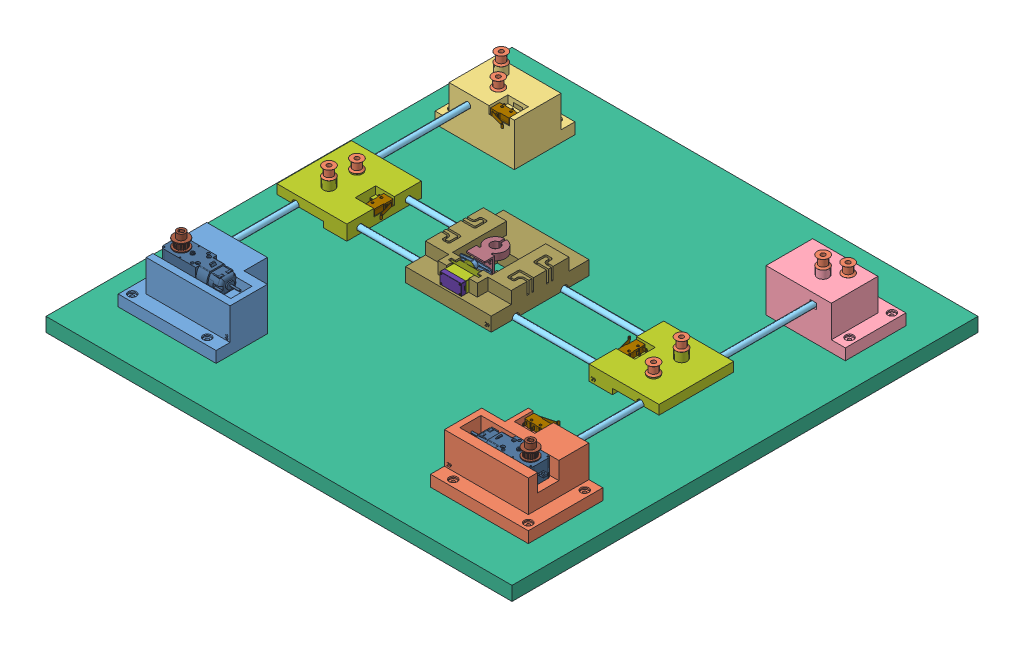
SolidWorks assembly LATEST ASSEMBLY, configuration Default. Lengths in mm.
Overall size (500 85.8 500).
74 component instances, 40 part files, 223 mates.
Components (placement in the parent):
- Stepper LEFT-2: Stepper LEFT [Default] at (56.9106 18.8224 107.4088) x (0 0 1) z (0 1 0) size (80 105 46)
- Stepper Right-1: Stepper Right [Default] at (296.9106 18.8224 42.4088) size (105 46 80)
- EndEffector 2-1: EndEffector 2 [Default] at (-28.0894 18.8224 -267.5912) size (85 56 65)
- EndEffector 1-1: EndEffector 1 [Default] at (384.024 18.8224 -217.5912) x (0 0 1) z (-1 0 0) size (65 54.7 85)
- Shaft-1: Shaft [Default] at (-8.0894 53.8224 -237.5912) x (-0.999824 -0.018749 0) z (-0.018749 0.999824 0) size (6 300 6)
- Shaft-4: Shaft [Default] at (361.9106 53.6724 -237.5912) x (-0.560083 -0.828436 0) z (-0.828436 0.560083 0) size (6 300 6)
- Base-2: Base [Default] at (426.9106 3.8224 -330.0912) size (500 15 500)
- END EFFECTOR 1-1: END EFFECTOR 1 [Default] at (321.9104 53.0886 -32.8378) x (0 0 -1) z (1 -0.000405 0) size (80 26 75)
- LMU-N6-1: LMU-N6 [Default] at (361.9106 53.6724 -72.5878) x (0 1 0) z (-1 0 0) size (12 19 12)
- END EFFECTOR 1-2: END EFFECTOR 1 [Default] at (31.9104 53.2062 -112.8378) x (0 0 1) z (-1 0.000405 0) size (80 26 75)
- LMU-N6-2: LMU-N6 [Default] at (-8.0894 53.8224 -73.0878) x (1 0 0) z (0 -1 0) size (12 19 12)
- Shaft-5: Shaft [Default] at (326.9104 53.0866 -98.8378) x (0.000405 1 0) z (0 0 1) size (6 300 6)
- Shaft-6: Shaft [Default] at (26.9104 53.2082 -46.8378) x (0.000401 0.988771 0.149436) z (0.000061 0.149436 -0.988771) size (6 300 6)
- LMU-N6-3: LMU-N6 [Default] at (167.865 53.151 -98.8378) x (0.000405 1 0) z (0 0 1) size (12 19 12)
- LMU-N6-4: LMU-N6 [Default] at (191.865 53.1413 -46.8378) x (0 0 -1) z (-0.000405 -1 0) size (12 19 12)
- LMU-N6-5: LMU-N6 [Default] at (145.865 53.16 -46.8378) x (0 0 -1) z (-0.000405 -1 0) size (12 19 12)
- A4_paper-1: A4_paper [Default] at (181.5617 18.8224 -76.6394) size (210 0.3 297) (hidden)
- SS_5GL13.step-10: SS_5GL13.step [Default] at (39.2125 58.4032 -68.0878) x (0 0 1) z (0.000405 1 0) size (21.03 22.89 6.4)
- SS_5GL13.step-11: SS_5GL13.step [Default] at (314.6125 58.2916 -77.5878) x (0 0 -1) z (0.000405 1 0) size (21.03 22.89 6.4)
- SS_5GL13.step-12: SS_5GL13.step [Default] at (337.6606 60.0224 50.1088) x (1 0 0) z (0 1 0) size (21.03 22.89 6.4)
- DG01D Motor-10: DG01D Motor [Default] at (-9.0894 55.8224 88.8088) x (-1 0 0) z (0 -1 0) size (79.2 22.5 37.6)
- DG01D Motor-11: DG01D Motor [Default] at (362.9106 46.0224 86.0088) x (1 0 0) z (0 -1 0) size (79.2 22.5 37.6)
- GT2 20T motor-2: GT2 20T motor [Default] at (-9.0894 83.1224 88.8088) x (0.422618 0 0.906308) z (0 1 0) size (16 16 15)
- GT2 20T motor-3: GT2 20T motor [Default] at (362.9106 73.3224 86.0088) x (-0.422618 0 -0.906308) z (0 1 0) size (16 16 15)
- belt Red^LATEST ASSEMBLY-1: belt Red^LATEST ASSEMBLY [Default] at origin (suppressed, hidden, virtual)
- SS_5GL13.step-14: SS_5GL13.step [Default] at (30.6606 60.0224 -225.2912) x (1 0 0) z (0 -1 0) size (21.03 22.89 6.4)
- ENDEFFECTOR-2: ENDEFFECTOR [Default] at (122.3648 52.6695 -125.3378) x (0 0 1) z (-1 0.000405 0) size (105 28 92)
- Pen Holder-2: Pen Holder [Default] at (168.2252 78.3723 -70.9178) x (0 0 1) z (0.000405 1 0) size (32.33 22 45.5)
- servo-3: servo [Default] at (161.2865 54.9158 -21.6708) x (1 -0.000405 0) z (0.000405 1 0) size (38.91 33.08 16.81)
  - servo.STEP-1: servo.STEP [Default] at origin size (38.91 33.08 16.81)
    - gear_sub1.STEP-1: gear_sub1.STEP [Default] at (5.1357 15.652 26.5654) x (-0.68795 0 -0.725758) z (0.725758 0 -0.68795) size (14.38 10.78 14.37)
      - scrow.STEP-1: scrow.STEP [Default] at (3.6352 0.49 7.5429) size (1 10.78 1)
      - spur gear_iso_ISO - Spur gear 0.25M 39T 20PA 1FW ---S39A75H50L1.0N.STEP-1: spur gear_iso_ISO - Spur gear 0.25M 39T 20PA 1FW ---S39A75H50L1.0N.STEP [Default] at (3.6352 0.49 7.5429) x (0 1 0) z (-0.789182 0 0.61416) size (1 10.24 10.25)
      - spur gear_iso_ISO - Spur gear 0.25M 10T 20PA 1.75FW ---S10A75H50L1.0N.STEP-1: spur gear_iso_ISO - Spur gear 0.25M 10T 20PA 1.75FW ---S10A75H50L1.0N.STEP [Default] at (3.6352 1.49 7.5429) x (0 1 0) z (-0.998551 0 0.053813) size (1.75 2.87 3)
    - gear_sub2.STEP-1: gear_sub2.STEP [Default] at (8.1037 16.927 13.0282) x (0.29675 0 0.954955) z (-0.954955 0 0.29675) size (10.78 2.75 10.78)
      - spur gear_iso_ISO - Spur gear 0.25M 39T 20PA 1FW ---S39A75H50L1.0N.STEP-1: spur gear_iso_ISO - Spur gear 0.25M 39T 20PA 1FW ---S39A75H50L1.0N.STEP [Default] at (3.6352 0.59 7.5429) x (0 1 0) z (-0.998551 0 0.053813) size (1 10.24 10.25)
      - spur gear_iso_ISO - Spur gear 0.25M 10T 20PA 1.75FW ---S10A75H50L1.0N.STEP-1: spur gear_iso_ISO - Spur gear 0.25M 10T 20PA 1.75FW ---S10A75H50L1.0N.STEP [Default] at (3.6352 1.59 7.5429) x (0 1 0) z (-0.998551 0 0.053813) size (1.75 2.87 3)
    - gear_sub3.STEP-1: gear_sub3.STEP [Default] at (15.6535 19.4558 12.7337) x (0.175743 0 0.984436) z (-0.984436 0 0.175743) size (10.78 7 10.78)
      - spur gear_iso_ISO - Spur gear 0.25M 39T 20PA 1FW ---S39A75H50L1.0N.STEP-1: spur gear_iso_ISO - Spur gear 0.25M 39T 20PA 1FW ---S39A75H50L1.0N.STEP [Default] at (4.585 -0.5638 8.482) x (0 1 0) z (-0.998551 0 0.053813) size (1 10.24 10.25)
      - spur gear_iso_ISO - Spur gear 0.25M 10T 20PA 6FW ---S10A75H50L1.0N.STEP-1: spur gear_iso_ISO - Spur gear 0.25M 10T 20PA 6FW ---S10A75H50L1.0N.STEP [Default] at (4.585 6.4362 8.482) x (0 -1 0) z (-0.985477 0 0.169808) size (6 2.87 3)
    - DcMotor Emsamblaje Final_Predeterminado.STEP-1: DcMotor Emsamblaje Final_Predeterminado.STEP [Default] at (14.2292 7.0834 18.738) x (0 0 1) z (0 1 0) size (9.11 7.45 12.63)
      - TapaCarcasaDcMotor_Predeterminado.STEP-1: TapaCarcasaDcMotor_Predeterminado.STEP [Default] at origin size (9.07 6.88 5)
      - RondanaDcMotor_Predeterminado.STEP-1: RondanaDcMotor_Predeterminado.STEP [Default] at (0 0 -4.154) x (-0.908878 0.417062 0) z (0 0 1) size (2.73 2.73 1.36)
      - Soportede Cobre_Predeterminado.STEP-1: Soportede Cobre_Predeterminado.STEP [Default] at (-2.4158 -0.0897 0.8236) x (-1 0 0) z (0 0 -1) size (3.11 2.85 3.19)
      - CarcasaDcMotor_Predeterminado.STEP-1: CarcasaDcMotor_Predeterminado.STEP [Default] at (-0.0001 -0.0021 2.4378) size (9.11 7.45 9.44)
      - Arcometalico_Predeterminado.STEP-1: Arcometalico_Predeterminado.STEP [Default] at (0 3.5144 -4.5886) x (1 0 0) z (0 0 -1) size (3.87 0.45 7.17)
      - AislanteDcMotor_Predeterminado.STEP-1: AislanteDcMotor_Predeterminado.STEP [Default] at (-4.0652 -0.1559 -3.4215) x (0.999266 0.038313 0) z (0 0 1) size (2.31 6.27 5.47)
      - AislanteDcMotor_Predeterminado.STEP-2: AislanteDcMotor_Predeterminado.STEP [Default] at (4.0652 -0.1559 8.5785) x (-0.999266 0.038313 0) z (0 0 -1) size (2.31 6.27 5.47)
      - Rondana2DcMotor_Predeterminado.STEP-1: Rondana2DcMotor_Predeterminado.STEP [Default] at (0 0 8.6961) x (-0.478461 0.878109 0) z (0 0 -1) size (2.5 2.5 0.8)
      - Soportede Cobre_Predeterminado.STEP-2: Soportede Cobre_Predeterminado.STEP [Default] at (2.4158 0.0897 0.8236) x (1 0 0) z (0 0 -1) size (3.11 2.85 3.19)
    - serv.Part4.STEP-1: serv.Part4.STEP [Default] at (-4.0208 15.6669 12.738) x (1 0 0) z (0 0 -1) size (23 11.2 12)
    - serv.Part1_2.STEP-1: serv.Part1_2.STEP [Default] at (-4.9734 17.9768 13.1998) x (0 0 1) z (1 0 0) size (9.5 4.83 9.5)
    - serv.Part2.STEP-1: serv.Part2.STEP [Default] at (1.9792 11.6669 18.738) x (0 1 0) z (-0.361678 0 0.932303) size (14 8.25 8.85)
    - serv.Part1_1.STEP-1: serv.Part1_1.STEP [Default] at (7.5718 13.1764 20.0943) x (-0.577909 -0.633022 0.515077) z (-0.311275 0.754407 0.577909) size (1.52 1.84 1.6)
    - gear_sub4.STEP-1: gear_sub4.STEP [Default] at (9.0139 24.755 13.5968) x (0 1 0) z (-0.779324 0 0.626621) size (7.5 10.24 10.25)
    - serv.Part8.STEP-1: serv.Part8.STEP [Default] at (3.3608 8.6863 18.738) x (0.906308 0.422618 0) z (0 0 -1) size (10 2.25 9)
    - wire^servo.STEP-1: wire^servo.STEP [Default] at origin size (1.78 1.52 7.94)
    - spur gear_iso_ISO - Spur gear 0.25M 10T 20PA 2FW ---S10A75H50L1.0N.STEP-1: spur gear_iso_ISO - Spur gear 0.25M 10T 20PA 2FW ---S10A75H50L1.0N.STEP [Default] at (14.2292 15.6419 18.738) x (0 1 0) z (0.11683 0 0.993152) size (2 2.87 3)
    - Rotor_Predeterminado.STEP-1: Rotor_Predeterminado.STEP [Default] at (14.2292 10.7797 18.738) x (0.046043 0 0.998939) z (0 1 0) size (5.79 5.7 16.91)
    - serv.Part5.STEP-1: serv.Part5.STEP [Default] at (-4.0208 15.6669 24.738) size (32 11 12.02)
    - serv.Part3.STEP-1: serv.Part3.STEP [Default] at (18.9792 0.6669 12.738) x (-1 0 0) z (0 1 0) size (23 12 5)
    - serv.Part6.STEP-1: serv.Part6.STEP [Default] at (17.7292 0.3169 23.488) x (0 1 0) z (0 0 1) size (20 2 2)
    - serv.Part6.STEP-2: serv.Part6.STEP [Default] at (-2.7708 0.3169 23.488) x (0 1 0) z (0.837169 0 0.546944) size (20 2 2)
    - serv.Part6.STEP-3: serv.Part6.STEP [Default] at (17.7292 0.3169 13.988) x (0 1 0) z (0.837169 0 0.546944) size (20 2 2)
    - serv.Part6.STEP-4: serv.Part6.STEP [Default] at (-2.7708 0.3169 13.988) x (0 1 0) z (0.6 0 0.8) size (20 2 2)
    - serv.Part7 servo hourn .STEP-1: serv.Part7 servo hourn .STEP [Default] at (-12.7504 33.3919 17.962) x (0.052604 0 -0.998615) z (0 -1 0) size (6.91 34.5 5)
- Pully-1: Pully [Default] at (351.2106 78.5224 -239.5912) x (1 0 0.000755) z (-0.000755 0 1) size (12.7 10 12.7)
- Pully-2: Pully [Default] at (363.0606 69.8224 -254.5912) size (12.7 10 12.7)
- Pully-3: Pully [Default] at (351.0705 78.0768 -87.8378) x (0.936747 -0.00038 -0.350007) z (0.350007 -0.000142 0.936747) size (12.7 10 12.7)
- Pully-4: Pully [Default] at (351.0671 69.6768 -57.8378) x (1 -0.000405 0) z (0 0 1) size (12.7 10 12.7)
- Pully-5: Pully [Default] at (-9.0894 79.8224 -254.5912) x (0.992904 0 -0.118917) z (0.118917 0 0.992904) size (12.7 10 12.7)
- Pully-6: Pully [Default] at (2.7606 69.8224 -239.5912) size (12.7 10 12.7)
- Pully-7: Pully [Default] at (2.7671 69.818 -87.8378) x (1 -0.000405 0) z (0 0 1) size (12.7 10 12.7)
- Pully-8: Pully [Default] at (2.7705 78.218 -57.8378) x (0.99977 -0.000405 0.021432) z (-0.021432 0.000009 0.99977) size (12.7 10 12.7)
Mates (geometry in assembly coordinates):
- Concentric1: concentric anti-aligned: cylinder of EndEffector 2-1 through (-8.0894 53.8224 -237.5912) axis (0 0 1) radius 3.15; cylinder of Shaft-1 through (-8.0894 53.8224 62.4088) axis (0 0 -1) radius 3
- Coincident1: coincident anti-aligned: plane of EndEffector 2-1 through (-8.0894 53.8224 -237.5912) normal (0 0 1); plane of Shaft-1 through (-8.0894 53.8224 -237.5912) normal (0 0 -1)
- Concentric2: concentric aligned: cylinder of Stepper LEFT-2 through (-8.0894 53.8224 62.4088) axis (0 0 -1) radius 3.2; cylinder of Shaft-1 through (-8.0894 53.8224 62.4088) axis (0 0 -1) radius 3
- Coincident2: coincident anti-aligned: plane of Stepper LEFT-2 through (-8.0894 53.8224 62.4088) normal (0 0 -1); plane of Shaft-1 through (-8.0894 53.8224 62.4088) normal (0 0 1)
- Concentric3: concentric aligned: cylinder of Stepper LEFT-2 through (22.0606 53.8224 74.9088) axis (1 0 0) radius 3.15; cylinder of Shaft-2 through (22.0606 53.8224 74.9088) axis (1 0 0) radius 3
- Coincident3: coincident anti-aligned: plane of Stepper LEFT-2 through (22.0606 53.8224 74.9088) normal (1 0 0); plane of Shaft-2 through (22.0606 53.8224 74.9088) normal (-1 0 0)
- Concentric4: concentric anti-aligned: cylinder of Stepper Right-1 through (322.0606 53.8224 74.9088) axis (-1 0 0) radius 3.15; cylinder of Shaft-2 through (22.0606 53.8224 74.9088) axis (1 0 0) radius 3
- Symmetric1: symmetric anti-aligned: plane of Stepper Right-1 through (322.0606 53.8224 74.9088) normal (-1 0 0); plane of Stepper Right-1 through (322.0606 53.8224 74.9088) normal (1 0 0); plane of Shaft-2 through (292.0606 64.8224 62.4088) normal (0 1 0)
- Concentric5: concentric: cylinder of EndEffector 2-1 through (22.0606 53.8224 -242.5912) axis (1 0 0) radius 3.15; cylinder of Shaft-3 through (22.0606 53.8224 -242.5912) axis (1 0 0) radius 3
- Coincident4: coincident: plane of EndEffector 2-1 through (22.0606 53.8224 -242.5912) normal (1 0 0); plane of Shaft-3 through (22.0606 53.8224 -242.5912) normal (-1 0 0)
- Concentric6: concentric: cylinder of EndEffector 1-1 through (322.0606 53.8224 -242.5912) axis (-1 0 0) radius 3.15; cylinder of Shaft-3 through (22.0606 53.8224 -242.5912) axis (1 0 0) radius 3
- Coincident5: coincident: plane of EndEffector 1-1 through (322.0606 53.8224 -242.5912) normal (-1 0 0); plane of Shaft-3 through (322.0606 53.8224 -242.5912) normal (1 0 0)
- Coincident6: coincident anti-aligned: plane of EndEffector 1-1 through (384.024 18.8224 -237.5912) normal (0 0 1); plane of Shaft-4 through (361.9106 53.6724 -237.5912) normal (0 0 -1)
- Coincident7: coincident anti-aligned: plane of Stepper Right-1 through (361.9106 53.8224 62.4088) normal (0 0 -1); plane of Shaft-4 through (361.9106 53.6724 62.4088) normal (0 0 1)
- Coincident14: coincident aligned: plane of Stepper LEFT-2 through (56.9106 18.8224 107.4088) normal (0 -1 0); plane of EndEffector 2-1 through (-28.0894 18.8224 -267.5912) normal (0 -1 0)
- Coincident15: coincident aligned: plane of Stepper LEFT-2 through (56.9106 18.8224 107.4088) normal (0 -1 0); plane of EndEffector 1-1 through (384.024 18.8224 -217.5912) normal (0 -1 0)
- Coincident16: coincident aligned: plane of Stepper LEFT-2 through (56.9106 18.8224 107.4088) normal (0 -1 0); plane of Stepper Right-1 through (296.9106 18.8224 42.4088) normal (0 -1 0)
- Coincident22: coincident anti-aligned: plane of Stepper Right-1 through (296.9106 18.8224 42.4088) normal (0 -1 0); plane of Base-2 through (426.9106 18.8224 -330.0912) normal (0 1 0)
- Distance4: distance = 30 mm aligned: plane of Stepper Right-1 through (396.9106 18.8224 42.4088) normal (1 0 0); plane of Base-2 through (426.9106 18.8224 -330.0912) normal (1 0 0)
- Concentric8: concentric aligned: cylinder of END EFFECTOR 1-1 through (361.9106 53.6724 -82.5878) axis (0 0 1) radius 6.2; cylinder of LMU-N6-1 through (361.9106 53.6724 -82.0878) axis (0 0 1) radius 6
- Coincident23: coincident anti-aligned: plane of END EFFECTOR 1-1 through (361.9106 53.6724 -63.0878) normal (0 0 -1); plane of LMU-N6-1 through (361.9106 53.6724 -63.0878) normal (0 0 1)
- Concentric9: concentric anti-aligned: cylinder of Shaft-4 through (361.9106 53.6724 62.4088) axis (0 0 -1) radius 3; cylinder of LMU-N6-1 through (361.9106 53.6724 -82.0878) axis (0 0 1) radius 3
- Concentric10: concentric aligned: cylinder of END EFFECTOR 1-2 through (-8.0894 53.8224 -63.0878) axis (0 0 -1) radius 6.2; cylinder of LMU-N6-2 through (-8.0894 53.8224 -63.5878) axis (0 0 -1) radius 6
- Coincident24: coincident anti-aligned: plane of END EFFECTOR 1-2 through (-8.0894 53.8224 -82.5878) normal (0 0 1); plane of LMU-N6-2 through (-8.0894 53.8224 -82.5878) normal (0 0 -1)
- Concentric11: concentric aligned: cylinder of Shaft-1 through (-8.0894 53.8224 62.4088) axis (0 0 -1) radius 3; cylinder of LMU-N6-2 through (-8.0894 53.8224 -63.5878) axis (0 0 -1) radius 3
- Concentric12: concentric anti-aligned: cylinder of END EFFECTOR 1-1 through (326.9104 53.0866 -98.8378) axis (-1 0.000405 0) radius 3.15; cylinder of Shaft-5 through (26.9104 53.2082 -98.8378) axis (1 -0.000405 0) radius 3
- Coincident25: coincident anti-aligned: plane of END EFFECTOR 1-2 through (26.9104 53.2082 -98.8378) normal (1 -0.000405 0); plane of Shaft-5 through (26.9104 53.2082 -98.8378) normal (-1 0.000405 0)
- Concentric13: concentric aligned: cylinder of END EFFECTOR 1-2 through (26.9104 53.2082 -98.8378) axis (1 -0.000405 0) radius 3.15; cylinder of Shaft-5 through (26.9104 53.2082 -98.8378) axis (1 -0.000405 0) radius 3
- Concentric14: concentric aligned: cylinder of END EFFECTOR 1-1 through (326.9104 53.0866 -46.8378) axis (-1 0.000405 0) radius 3.15; cylinder of Shaft-6 through (326.9104 53.0866 -46.8378) axis (-1 0.000405 0) radius 3
- Coincident26: coincident anti-aligned: plane of END EFFECTOR 1-2 through (26.9104 53.2082 -46.8378) normal (1 -0.000405 0); plane of Shaft-6 through (26.9104 53.2082 -46.8378) normal (-1 0.000405 0)
- Concentric15: concentric aligned: cylinder of EndEffectorBase-1 through (152.1321 53.2224 -24.3407) axis (1 0 0) radius 6; cylinder of LMU-N6-3 through (158.365 53.1549 -98.8378) axis (1 -0.000405 0) radius 6
- Coincident27: coincident anti-aligned: plane of EndEffectorBase-1 through (109.2714 53.2224 51.6596) normal (-1 0 0); plane of LMU-N6-3 through (177.365 53.1472 -98.8378) normal (1 -0.000405 0)
- Concentric16: concentric anti-aligned: cylinder of EndEffectorBase-1 through (152.1321 53.2224 27.6593) axis (1 0 0) radius 6; cylinder of LMU-N6-4 through (201.365 53.1375 -46.8378) axis (-1 0.000405 0) radius 6
- Coincident28: coincident anti-aligned: plane of EndEffectorBase-1 through (130.0583 53.2224 51.6596) normal (-1 0 0); plane of LMU-N6-4 through (201.365 53.1375 -46.8378) normal (1 -0.000405 0)
- Concentric17: concentric anti-aligned: cylinder of EndEffectorBase-1 through (152.1321 53.2224 27.6593) axis (1 0 0) radius 6; cylinder of LMU-N6-5 through (155.365 53.1561 -46.8378) axis (-1 0.000405 0) radius 6
- Coincident29: coincident anti-aligned: plane of EndEffectorBase-1 through (68.9844 53.2224 51.6596) normal (1 0 0); plane of LMU-N6-5 through (136.365 53.1638 -46.8378) normal (-1 0.000405 0)
- Concentric18: concentric aligned: cylinder of Shaft-5 through (26.9104 53.2082 -98.8378) axis (1 -0.000405 0) radius 3; cylinder of LMU-N6-3 through (158.365 53.1549 -98.8378) axis (1 -0.000405 0) radius 3
- Concentric19: concentric aligned: cylinder of Shaft-6 through (326.9104 53.0866 -46.8378) axis (-1 0.000405 0) radius 3; cylinder of LMU-N6-4 through (201.365 53.1375 -46.8378) axis (-1 0.000405 0) radius 3
- Coincident30: coincident anti-aligned: plane of Stepper LEFT-2 through (52.0606 62.0224 127.4088) normal (0 -1 0); plane of DG01D Motor-1 through (-6.752 62.0224 108.4088) normal (0 1 0)
- Concentric20: concentric anti-aligned: cylinder of Stepper LEFT-2 through (-13.8394 91.0224 107.4088) axis (0 -1 0) radius 3.25; cylinder of DG01D Motor-1 through (-13.8394 71.4192 107.4088) axis (0 1 0) radius 1.2093
- Parallel5: parallel anti-aligned: plane of Stepper LEFT-2 through (55.5106 62.0224 100.1588) normal (-1 0 0); plane of DG01D Motor-1 through (39.1606 62.1259 108.3931) normal (1 0 0)
- Coincident33: coincident anti-aligned: plane of Stepper Right-1 through (292.0606 62.0224 62.4088) normal (0 -1 0); plane of DG01D Motor-2 through (350.8733 62.0224 106.1057) normal (0 1 0)
- Concentric21: concentric anti-aligned: cylinder of Stepper Right-1 through (357.9606 105.2224 107.1057) axis (0 -1 0) radius 3.25; cylinder of DG01D Motor-2 through (357.9606 71.4192 107.1057) axis (0 1 0) radius 1.2093
- Parallel6: parallel anti-aligned: plane of Stepper Right-1 through (298.3106 62.0224 74.6588) normal (1 0 0); plane of DG01D Motor-2 through (304.9606 62.1259 106.1214) normal (-1 0 0)
- Coincident38: coincident anti-aligned: plane of EndEffector 1-1 through (382.0606 64.8224 -217.5912) normal (0 0 1); plane of SS_5GL13.step-1 through (374.976 62.6859 -217.5912) normal (0 0 -1)
- Coincident39: coincident anti-aligned: plane of Stepper LEFT-2 through (56.9106 64.8224 42.4088) normal (0 0 -1); plane of SS_5GL13.step-2 through (14.4666 56.8442 62.4088) normal (0 0 1)
- Coincident40: coincident: plane of Stepper LEFT-2 through (56.9106 64.8224 42.4088) normal (0 0 -1); plane of SS_5GL13.step-3 through (-25.8206 63.4371 62.4088) normal (0 0 1)
- Concentric23: concentric: cylinder of DG01D Motor-2 through (357.9606 71.4192 107.1057) axis (0 1 0) radius 1.2093; cylinder of gear_pulley_V2.stp-1 through (332.7387 88.3224 3421.9714) axis (0 1 0) radius 1.8
- Concentric24: concentric: cylinder of DG01D Motor-2 through (357.9606 52.6192 107.1057) axis (0 1 0) radius 2.6; cylinder of gear_pulley_V2.stp-1 through (332.7387 69.8224 3421.9714) axis (0 -1 0) radius 2.8
- Parallel9: parallel: plane of DG01D Motor-2 through (355.5058 33.8192 106.2489) normal (-0.422618 0 -0.906308); plane of gear_pulley_V2.stp-1 through (330.7791 69.8224 3423.9714) normal (0 0 -1)
- Coincident45: coincident anti-aligned: plane of Stepper Right-1 through (296.9106 64.8224 42.4088) normal (0 1 0); plane of gear_pulley_V2.stp-1 through (332.7387 64.8224 3421.9714) normal (0 -1 0)
- Concentric25: concentric aligned: cylinder of DG01D Motor-1 through (-13.8394 71.4192 107.4088) axis (0 1 0) radius 1.2093; cylinder of gear_pulley_V2.stp-2 through (-8.9394 88.3224 87.4088) axis (0 1 0) radius 1.8
- Coincident46: coincident anti-aligned: plane of Stepper LEFT-2 through (56.9106 64.8224 107.4088) normal (0 1 0); plane of gear_pulley_V2.stp-2 through (-8.9394 64.8224 87.4088) normal (0 -1 0)
- Coincident59: coincident anti-aligned: plane of DG01D Motor-2 through (350.8733 43.2224 108.1057) normal (0 -1 0); plane of Stepper base 2-1 through (293.4606 43.2224 94.9588) normal (0 1 0)
- Coincident60: coincident anti-aligned: plane of Stepper Right-1 through (298.3106 62.0224 97.3588) normal (0 0 -1); plane of Stepper base 2-1 through (293.4606 43.2224 120.1588) normal (0 0 1)
- Coincident61: coincident anti-aligned: plane of Stepper Right-1 through (298.3106 62.0224 74.6588) normal (1 0 0); plane of Stepper base 2-1 through (293.4606 43.2224 94.9588) normal (-1 0 0)
- Coincident64: coincident anti-aligned: plane of DG01D Motor-1 through (-6.752 43.2224 106.4088) normal (0 -1 0); plane of Stepper base 1-2 through (50.6606 43.2224 119.8588) normal (0 1 0)
- Coincident65: coincident anti-aligned: plane of Stepper LEFT-2 through (55.5106 62.0224 100.1588) normal (-1 0 0); plane of Stepper base 1-2 through (50.6606 43.2224 119.8588) normal (1 0 0)
- Coincident66: coincident anti-aligned: plane of Stepper LEFT-2 through (55.5106 62.0224 77.4588) normal (0 0 1); plane of Stepper base 1-2 through (50.6606 43.2224 94.6588) normal (0 0 -1)
- Coincident68: coincident anti-aligned: plane of END EFFECTOR 1-2 through (32.0606 61.6224 -45.5396) normal (0 -1 0); plane of SS_5GL13.step-4 through (21.8606 61.6224 -45.9396) normal (0 1 0)
- Coincident69: coincident anti-aligned: plane of END EFFECTOR 1-2 through (32.0606 61.6224 -65.7396) normal (0 0 1); plane of SS_5GL13.step-4 through (21.8606 61.6224 -65.7396) normal (0 0 -1)
- Coincident71: coincident aligned: plane of END EFFECTOR 1-2 through (46.9104 53.2001 -46.8378) normal (1 -0.000405 0); plane of SS_5GL13.step-4 through (32.0606 61.6224 -65.7396) normal (1 0 0)
- Coincident72: coincident anti-aligned: plane of END EFFECTOR 1-1 through (312.0606 61.6224 -65.7396) normal (0 -1 0); plane of SS_5GL13.step-5 through (321.5606 61.6224 -65.3396) normal (0 1 0)
- Coincident73: coincident anti-aligned: plane of END EFFECTOR 1-1 through (312.0606 61.6224 -45.5396) normal (0 0 -1); plane of SS_5GL13.step-5 through (321.5606 61.6224 -45.5396) normal (0 0 1)
- Coincident74: coincident aligned: plane of END EFFECTOR 1-1 through (306.9104 53.0947 -98.8378) normal (-1 0.000405 0); plane of SS_5GL13.step-5 through (312.0606 61.6224 -55.2396) normal (-1 0 0)
- Coincident75: coincident anti-aligned: plane of END EFFECTOR 1-1 through (365.3606 61.6224 -0.6396) normal (0 -1 0); plane of SS_5GL13.step-6 through (365.7606 61.6224 -10.1396) normal (0 1 0)
- Coincident76: coincident anti-aligned: plane of END EFFECTOR 1-1 through (385.5606 61.6224 -0.6396) normal (-1 0 0); plane of SS_5GL13.step-6 through (385.5606 61.6224 -10.1396) normal (1 0 0)
- Coincident77: coincident aligned: plane of END EFFECTOR 1-1 through (327.0606 53.2224 -0.6396) normal (0 0 1); plane of SS_5GL13.step-6 through (375.8606 61.6224 -0.6396) normal (0 0 1)
- Coincident78: coincident anti-aligned: plane of END EFFECTOR 1-2 through (-21.2394 61.6224 -110.6396) normal (0 -1 0); plane of SS_5GL13.step-7 through (-21.6394 61.6224 -101.1396) normal (0 1 0)
- Coincident79: coincident anti-aligned: plane of END EFFECTOR 1-2 through (-41.4394 61.6224 -110.6396) normal (1 0 0); plane of SS_5GL13.step-7 through (-41.4394 61.6224 -101.1396) normal (-1 0 0)
- Coincident80: coincident aligned: plane of END EFFECTOR 1-2 through (17.0606 53.2224 -110.6396) normal (0 0 -1); plane of SS_5GL13.step-7 through (-31.7394 61.6224 -110.6396) normal (0 0 -1)
- Coincident81: coincident anti-aligned: plane of Base-2 through (426.9106 18.8224 -330.0912) normal (0 1 0); plane of A4_paper-1 through (181.5617 18.8224 -76.6394) normal (0 -1 0)
- Coincident82: coincident anti-aligned: plane of END EFFECTOR 1-2 through (26.9112 55.2082 -61.8378) normal (0.000405 1 0); plane of SS_5GL13.step-8 through (34.4996 55.2224 -80.2) normal (0 -1 0)
- Coincident84: coincident aligned: plane of END EFFECTOR 1-2 through (46.9104 53.2001 -46.8378) normal (1 -0.000405 0); plane of SS_5GL13.step-9 through (32.0606 61.6224 -84.8644) normal (1 0 0)
- Coincident85: coincident anti-aligned: plane of END EFFECTOR 1-2 through (26.9112 55.2082 -61.8378) normal (0.000405 1 0); plane of SS_5GL13.step-9 through (21.8606 55.2224 -65.0644) normal (0 -1 0)
- Concentric37: concentric aligned: cylinder of END EFFECTOR 1-2 through (39.2031 35.2032 -68.0878) axis (0.000405 1 0) radius 1.185; cylinder of SS_5GL13.step-10 through (39.2112 55.2032 -68.0878) axis (0.000405 1 0) radius 1.175
- Concentric38: concentric aligned: cylinder of END EFFECTOR 1-2 through (39.2031 35.2032 -77.5878) axis (0.000405 1 0) radius 1.185; cylinder of SS_5GL13.step-10 through (39.2112 55.2032 -77.5878) axis (0.000405 1 0) radius 1.25
- Coincident86: coincident anti-aligned: plane of END EFFECTOR 1-2 through (26.9112 55.2082 -61.8378) normal (0.000405 1 0); plane of SS_5GL13.step-10 through (36.7112 55.2042 -62.8878) normal (-0.000405 -1 0)
- Concentric39: concentric aligned: circle of END EFFECTOR 1-1; unknown of SS_5GL13.step-11
- Concentric40: concentric aligned: cylinder of END EFFECTOR 1-1; cylinder of SS_5GL13.step-11 through (314.6112 55.0916 -68.0878) axis (0.000405 1 0) radius 1.25
- Coincident88: coincident anti-aligned: plane of END EFFECTOR 1-1 through (326.9112 55.0866 -83.8378) normal (0.000405 1 0); plane of SS_5GL13.step-11 through (317.1112 55.0905 -82.7878) normal (-0.000405 -1 0)
- Concentric41: concentric aligned: cylinder of Stepper Right-1 through (328.1606 46.8224 50.1088) axis (0 1 0) radius 1.185; cylinder of SS_5GL13.step-12 through (328.1606 56.8224 50.1088) axis (0 1 0) radius 1.25
- Concentric42: concentric aligned: cylinder of Stepper Right-1 through (337.6606 46.8224 50.1088) axis (0 1 0) radius 1.185; cylinder of SS_5GL13.step-12 through (337.6606 56.8224 50.1088) axis (0 1 0) radius 1.175
- Coincident89: coincident anti-aligned: plane of Stepper Right-1 through (343.9106 56.8224 62.4088) normal (0 1 0); plane of SS_5GL13.step-12 through (342.8606 56.8224 52.6088) normal (0 -1 0)
- Concentric43: concentric aligned: cylinder of Stepper LEFT-2 through (25.8106 46.8224 50.1088) axis (0 1 0) radius 1.185; cylinder of SS_5GL13.step-13 through (25.8106 56.8224 50.1088) axis (0 1 0) radius 1.175
- Concentric44: concentric aligned: cylinder of Stepper LEFT-2 through (16.3106 46.8224 50.1088) axis (0 1 0) radius 1.185; cylinder of SS_5GL13.step-13 through (16.3106 56.8224 50.1088) axis (0 1 0) radius 1.25
- Coincident91: coincident anti-aligned: plane of Stepper LEFT-2 through (32.0606 56.8224 62.4088) normal (0 1 0); plane of SS_5GL13.step-13 through (31.0106 56.8224 52.6088) normal (0 -1 0)
- Concentric50: concentric anti-aligned: cylinder of Stepper LEFT-2 through (-9.0894 2.3724 88.8088) axis (0 1 0) radius 3.25; cylinder of DG01D Motor-4 through (-13.8394 36.4255 107.4088) axis (0 -1 0) radius 1.2093
- Concentric51: concentric anti-aligned: cylinder of Stepper LEFT-2 through (3.2106 2.3724 88.8088) axis (0 1 0) radius 2.35; cylinder of DG01D Motor-4 through (-1.5394 44.3382 107.4088) axis (0 -1 0) radius 0.5
- Coincident97: coincident anti-aligned: plane of Stepper LEFT-2 through (56.9106 55.8224 107.4088) normal (0 1 0); plane of DG01D Motor-4 through (-6.752 45.8224 106.4088) normal (0 -1 0)
- Concentric52: concentric anti-aligned: cylinder of Stepper LEFT-2 through (-9.0894 2.3724 88.8088) axis (0 1 0) radius 3.25; cylinder of DG01D Motor-5 through (-13.8394 36.4255 107.4088) axis (0 -1 0) radius 1.2093
- Concentric53: concentric aligned: cylinder of Stepper LEFT-2 through (3.2106 2.3724 88.8088) axis (0 1 0) radius 2.35; cylinder of DG01D Motor-5 through (-1.5394 45.0803 107.4088) axis (0 1 0) radius 1.9
- Coincident98: coincident anti-aligned: plane of Stepper LEFT-2 through (56.9106 55.8224 107.4088) normal (0 1 0); plane of DG01D Motor-5 through (-6.752 45.8224 106.4088) normal (0 -1 0)
- Concentric54: concentric anti-aligned: cylinder of DG01D Motor-5 through (-13.8394 36.4255 107.4088) axis (0 -1 0) radius 1.2093; cylinder of gear_pulley_V2.stp-4 through (363.0606 74.6224 87.4088) axis (0 1 0) radius 1.8
- Parallel10: parallel anti-aligned: plane of DG01D Motor-5 through (-12.9178 74.0255 109.8401) normal (-0.422618 0 0.906308); plane of gear_pulley_V2.stp-4 through (364.4989 56.1224 85.0065) normal (0.233559 0 0.972343)
- Tangent1: tangent anti-aligned: plane of DG01D Motor-5 through (-5.6314 74.0255 106.1995) normal (0 1 0); cylinder of gear_pulley_V2.stp-4 through (374.8542 62.6224 84.576) axis (-0.972343 0 0.233559) radius 2
- Concentric55: concentric anti-aligned: cylinder of Stepper Right-1 through (362.9106 19.0224 86.0088) axis (0 1 0) radius 3.25; cylinder of DG01D Motor-6 through (363.0606 22.9255 107.4088) axis (0 -1 0) radius 1.2093
- Concentric57: concentric aligned: cylinder of Stepper Right-1 through (350.6106 19.0224 86.0088) axis (0 1 0) radius 2.35; cylinder of DG01D Motor-6 through (350.7606 31.5803 107.4088) axis (0 1 0) radius 1.9
- Coincident102: coincident anti-aligned: plane of Stepper Right-1 through (296.9106 46.0224 42.4088) normal (0 1 0); plane of DG01D Motor-6 through (355.9733 32.3224 108.4088) normal (0 -1 0)
- Concentric60: concentric anti-aligned: cylinder of DG01D Motor-6 through (363.0606 22.9255 107.4088) axis (0 -1 0) radius 1.2093; cylinder of gear_pulley_V2.stp-6 through (644.2279 1514.2792 90.8272) axis (0 0 1) radius 1.8
- Parallel12: parallel aligned: plane of DG01D Motor-6 through (362.1391 60.5255 104.9776) normal (0.422618 0 -0.906308); plane of gear_pulley_V2.stp-6 through (646.1875 1516.2792 72.3272) normal (0 -1 0)
- Tangent2: tangent anti-aligned: plane of DG01D Motor-6 through (354.8526 60.5255 108.6182) normal (0 1 0); cylinder of gear_pulley_V2.stp-6 through (632.0988 1514.2792 78.8272) axis (1 0 0) radius 2
- Concentric65: concentric anti-aligned: cylinder of DG01D Motor-6 through (363.0606 22.9255 107.4088) axis (0 -1 0) radius 1.2093; cylinder of gear_pulley_V2.stp-5 through (363.0606 74.5255 107.4088) axis (0 1 0) radius 1.8
- Parallel13: parallel aligned: plane of DG01D Motor-6 through (362.1391 60.5255 104.9776) normal (0.422618 0 -0.906308); plane of gear_pulley_V2.stp-5 through (360.4394 56.0255 108.3933) normal (0.422618 0 -0.906308)
- Tangent3: tangent anti-aligned: plane of DG01D Motor-6 through (354.8526 60.5255 108.6182) normal (0 1 0); cylinder of gear_pulley_V2.stp-5 through (374.0533 62.5255 112.5348) axis (-0.906308 0 -0.422618) radius 2
- Coincident113: coincident anti-aligned: plane of Stepper LEFT-2 through (56.9106 55.8224 107.4088) normal (0 1 0); plane of DG01D Motor-9 through (-6.7637 45.8224 106.3297) normal (0 -1 0)
- Concentric70: concentric aligned: cylinder of Stepper LEFT-2; cylinder of DG01D Motor-9 through (-13.8394 74.0192 107.4088) axis (0 1 0) radius 1.2093
- Coincident115: coincident anti-aligned: plane of Stepper LEFT-2 through (56.9106 55.8224 107.4088) normal (0 1 0); plane of DG01D Motor-10 through (-2.002 55.8224 87.8088) normal (0 -1 0)
- Concentric74: concentric aligned: cylinder of Stepper LEFT-2 through (-9.0894 2.3724 88.8088) axis (0 1 0) radius 3.25; cylinder of DG01D Motor-10 through (-9.0894 84.0192 88.8088) axis (0 1 0) radius 1.2093
- Concentric75: concentric aligned: cylinder of Stepper LEFT-2 through (11.5106 2.3724 80.0588) axis (0 1 0) radius 1.5; cylinder of DG01D Motor-10 through (11.5106 46.4192 80.0588) axis (0 1 0) radius 1.5
- Concentric76: concentric aligned: cylinder of Stepper LEFT-2 through (11.5106 2.3724 97.5588) axis (0 1 0) radius 1.5; cylinder of DG01D Motor-10 through (11.5106 46.4192 97.5588) axis (0 1 0) radius 1.5
- Coincident116: coincident anti-aligned: plane of Stepper Right-1 through (296.9106 46.0224 42.4088) normal (0 1 0); plane of DG01D Motor-11 through (355.8233 46.0224 87.0088) normal (0 -1 0)
- Concentric77: concentric aligned: cylinder of Stepper Right-1 through (362.9106 19.0224 86.0088) axis (0 1 0) radius 3.25; cylinder of DG01D Motor-11 through (362.9106 74.2192 86.0088) axis (0 1 0) radius 1.2093
- Concentric78: concentric aligned: cylinder of Stepper Right-1 through (342.3106 19.0224 94.7588) axis (0 1 0) radius 1.5; cylinder of DG01D Motor-11 through (342.3106 36.6192 94.7588) axis (0 1 0) radius 1.5
- Concentric82: concentric aligned: cylinder of DG01D Motor-10 through (-9.0894 84.0192 88.8088) axis (0 1 0) radius 1.2093; cylinder of gear_pulley_V2.stp-2 through (-8.9394 88.3224 87.4088) axis (0 1 0) radius 1.8
- Coincident119: coincident anti-aligned: plane of DG01D Motor-11 through (355.8233 64.8224 85.0088) normal (0 1 0); plane of gear_pulley_V2.stp-4 through (363.0606 51.1224 87.4088) normal (0 -1 0)
- Concentric84: concentric aligned: cylinder of DG01D Motor-11 through (362.9106 74.2192 86.0088) axis (0 1 0) radius 1.2093; cylinder of gear_pulley_V2.stp-4 through (363.0606 74.6224 87.4088) axis (0 1 0) radius 1.8
- Distance9: distance = 47.5 mm aligned: plane of Base-2 through (426.9106 18.8224 -330.0912) normal (0 0 -1); plane of EndEffector 1-1 through (384.024 18.8224 -282.5912) normal (0 0 -1)
- Distance14: distance = 47.5 mm aligned: plane of Stepper LEFT-2 through (56.9106 18.8224 122.4088) normal (0 0 1); plane of Base-2 through (426.9106 18.8224 169.9088) normal (0 0 1)
- Coincident120: coincident anti-aligned: plane of END EFFECTOR 1-1 through (326.9104 53.0866 -98.8378) normal (-1 0.000405 0); plane of Shaft-5 through (326.9104 53.0866 -98.8378) normal (1 -0.000405 0)
- LimitDistance1: limit distance = 0 mm anti-aligned: plane of EndEffectorBase-1 through (46.9106 62.7098 -45.2346) normal (-1 0 0); plane of END EFFECTOR 1-2 through (46.9104 53.2001 -46.8378) normal (1 -0.000405 0)
- Concentric90: concentric aligned: cylinder of DG01D Motor-10 through (-9.0894 65.2192 88.8088) axis (0 1 0) radius 2.6; cylinder of GT2 20T motor-2 through (-9.0894 83.1224 88.8088) axis (0 1 0) radius 2.6
- Parallel15: parallel aligned: plane of DG01D Motor-10 through (-6.6346 46.4192 89.6656) normal (0.422618 0 0.906308); plane of GT2 20T motor-2 through (-9.8543 70.8067 87.1684) normal (0.422618 0 0.906308)
- Concentric91: concentric aligned: cylinder of DG01D Motor-10 through (-9.0894 65.2192 88.8088) axis (0 1 0) radius 2.6; cylinder of GT2 20T motor-2 through (-9.0894 83.1224 88.8088) axis (0 1 0) radius 2.6
- Coincident125: coincident anti-aligned: plane of DG01D Motor-10 through (-2.002 74.6224 89.8088) normal (0 1 0); plane of GT2 20T motor-2 through (-9.0894 74.6224 88.8088) normal (0 -1 0)
- Concentric92: concentric aligned: cylinder of DG01D Motor-11 through (362.9106 74.2192 86.0088) axis (0 1 0) radius 1.2093; cylinder of GT2 20T motor-3 through (362.9106 73.3224 86.0088) axis (0 1 0) radius 2.6
- Parallel16: parallel anti-aligned: plane of DG01D Motor-11 through (361.9891 36.6192 88.4401) normal (0.422618 0 0.906308); plane of GT2 20T motor-3 through (363.6755 61.0067 87.6493) normal (-0.422618 0 -0.906308)
- Coincident127: coincident anti-aligned: plane of DG01D Motor-11 through (355.8233 64.8224 85.0088) normal (0 1 0); plane of GT2 20T motor-3 through (355.6601 64.8224 89.3898) normal (0 -1 0)
- Concentric93: concentric aligned: cylinder of END EFFECTOR 1-1 through (351.0563 43.0768 -57.8378) axis (0.000405 1 0) radius 2.5; cylinder of GT2 20T pulley-1 through (351.0685 73.1768 -58.832) axis (0.000405 1 0) radius 2.625
- Coincident128: coincident anti-aligned: plane of END EFFECTOR 1-1 through (351.0651 64.6768 -57.8378) normal (0.000405 1 0); plane of GT2 20T pulley-1 through (355.4406 64.675 -65.5293) normal (-0.000405 -1 0)
- Concentric94: concentric aligned: cylinder of END EFFECTOR 1-1 through (351.0563 43.0768 -87.8378) axis (0.000405 1 0) radius 2.5; cylinder of GT2 20T pulley-2 through (351.0719 81.5768 -88.832) axis (0.000405 1 0) radius 2.625
- Coincident129: coincident anti-aligned: plane of END EFFECTOR 1-1 through (351.0685 73.0768 -87.8378) normal (0.000405 1 0); plane of GT2 20T pulley-2 through (355.444 73.075 -95.5293) normal (-0.000405 -1 0)
- Concentric95: concentric aligned: cylinder of EndEffector 1-1 through (363.0606 54.8224 -254.5912) axis (0 1 0) radius 2.5; cylinder of GT2 20T pulley-3 through (363.0606 73.3224 -254.5912) axis (0 1 0) radius 2.625
- Coincident130: coincident anti-aligned: plane of EndEffector 1-1 through (384.024 64.8224 -217.5912) normal (0 1 0); plane of GT2 20T pulley-3 through (367.4362 64.8224 -261.2885) normal (0 -1 0)
- Concentric96: concentric aligned: cylinder of EndEffector 1-1 through (351.2106 54.8224 -239.5912) axis (0 1 0) radius 2.5; cylinder of GT2 20T pulley-4 through (351.2106 82.0224 -239.5912) axis (0 1 0) radius 2.625
- Coincident131: coincident anti-aligned: plane of EndEffector 1-1 through (351.2106 73.5224 -239.5912) normal (0 1 0); plane of GT2 20T pulley-4 through (359.0759 73.5224 -241.0531) normal (0 -1 0)
- Concentric97: concentric aligned: cylinder of EndEffector 2-1 through (2.7606 54.8224 -239.5912) axis (0 1 0) radius 2.5; cylinder of GT2 20T pulley-5 through (2.7606 73.3224 -239.5912) axis (0 1 0) radius 2.625
- Coincident132: coincident anti-aligned: plane of EndEffector 2-1 through (-28.0894 64.8224 -267.5912) normal (0 1 0); plane of GT2 20T pulley-5 through (7.1362 64.8224 -246.2885) normal (0 -1 0)
- Concentric98: concentric aligned: cylinder of EndEffector 2-1 through (-9.0894 54.8224 -254.5912) axis (0 1 0) radius 2.5; cylinder of GT2 20T pulley-6 through (-9.0894 83.3224 -254.5912) axis (0 1 0) radius 2.625
- Coincident133: coincident anti-aligned: plane of EndEffector 2-1 through (-9.0894 74.8224 -254.5912) normal (0 1 0); plane of GT2 20T pulley-6 through (-4.7138 74.8224 -261.2885) normal (0 -1 0)
- Concentric99: concentric aligned: cylinder of END EFFECTOR 1-2 through (2.7563 43.218 -87.8378) axis (0.000405 1 0) radius 2.5; cylinder of GT2 20T pulley-7 through (2.7685 73.318 -88.832) axis (0.000405 1 0) radius 2.625
- Coincident134: coincident anti-aligned: plane of END EFFECTOR 1-2 through (2.7651 64.818 -87.8378) normal (0.000405 1 0); plane of GT2 20T pulley-7 through (7.1406 64.8162 -95.5293) normal (-0.000405 -1 0)
- Concentric100: concentric aligned: cylinder of END EFFECTOR 1-2 through (2.7563 43.218 -57.8378) axis (0.000405 1 0) radius 2.5; cylinder of GT2 20T pulley-8 through (2.7719 81.718 -58.832) axis (0.000405 1 0) radius 2.625
- Coincident135: coincident anti-aligned: plane of END EFFECTOR 1-2 through (2.7685 73.218 -57.8378) normal (0.000405 1 0); plane of GT2 20T pulley-8 through (4.21 73.2174 -66.701) normal (-0.000405 -1 0)
- InPlace1: in place: plane of ? through (363.0606 65.8224 86.0088) normal (0 1 0); plane of ? through (0 65.8224 0) normal (0 1 0); moOrthogonalPlaneRef_w of ? through (363.0606 65.8224 86.0088) normal (0 1 0); plane of ? through (0 65.8224 0) normal (0 0 -1); plane of ? through (363.0606 65.8224 86.0088) normal (0 1 0); plane of ? through (0 65.8224 0) normal (1 0 0); plane of GT2 20T motor-3 through (362.9106 65.8224 86.0088) normal (0 1 0); unknown of ?
- Coincident136: coincident aligned: plane of ?; plane of ?
- Coincident137: coincident aligned: plane of GT2 20T motor-3 through (362.9106 65.8224 86.0088) normal (-0.906308 0 0.422618); plane of Part1^LATEST ASSEMBLY-1 through (363.0606 65.8224 86.0088) normal (-0.906308 0 0.422618)
- Coincident138: coincident anti-aligned: plane of GT2 20T motor-3 through (362.9106 65.8224 86.0088) normal (0.422618 0 0.906308); plane of Part1^LATEST ASSEMBLY-1 through (363.0606 65.8224 86.0088) normal (-0.422618 0 -0.906308)
- InPlace2: in place: plane of ? through (363.0606 65.8224 86.0088) normal (0 1 0); plane of ? through (0 65.8224 0) normal (0 1 0); plane of ? through (363.0606 65.8224 86.0088) normal (0 1 0); plane of ? through (0 65.8224 0) normal (0 0 -1); plane of ? through (363.0606 65.8224 86.0088) normal (0 1 0); plane of ? through (0 65.8224 0) normal (1 0 0); plane of GT2 20T motor-3 through (362.9106 65.8224 86.0088) normal (0 1 0); unknown of ?
- Coincident139: coincident aligned: plane of ?; plane of ?
- Coincident140: coincident aligned: plane of GT2 20T motor-3 through (362.9106 65.8224 86.0088) normal (-0.906308 0 0.422618); plane of Part2^LATEST ASSEMBLY-1 through (363.0606 65.8224 86.0088) normal (-0.906308 0 0.422618)
- Coincident141: coincident anti-aligned: plane of GT2 20T motor-3 through (362.9106 65.8224 86.0088) normal (0.422618 0 0.906308); plane of Part2^LATEST ASSEMBLY-1 through (363.0606 65.8224 86.0088) normal (-0.422618 0 -0.906308)
- InPlace3: in place: plane of ? through (363.0606 65.8224 86.0088) normal (0 1 0); plane of ? through (0 65.8224 0) normal (0 1 0); plane of ? through (363.0606 65.8224 86.0088) normal (0 1 0); plane of ? through (0 65.8224 0) normal (0 0 -1); plane of ? through (363.0606 65.8224 86.0088) normal (0 1 0); plane of ? through (0 65.8224 0) normal (1 0 0); plane of GT2 20T motor-3 through (362.9106 65.8224 86.0088) normal (0 1 0); unknown of ?
- Coincident142: coincident aligned: plane of ?; plane of ?
- Coincident143: coincident aligned: plane of GT2 20T motor-3 through (362.9106 65.8224 86.0088) normal (-0.906308 0 0.422618); plane of Part3^LATEST ASSEMBLY-1 through (363.0606 65.8224 86.0088) normal (-0.906308 0 0.422618)
- Coincident144: coincident anti-aligned: plane of GT2 20T motor-3 through (362.9106 65.8224 86.0088) normal (0.422618 0 0.906308); plane of Part3^LATEST ASSEMBLY-1 through (363.0606 65.8224 86.0088) normal (-0.422618 0 -0.906308)
- InPlace4: in place: plane of ? through (366.4024 65.8224 -259.7063) normal (0 1 0); plane of ? through (0 65.8224 0) normal (0 1 0); plane of ? through (366.4024 65.8224 -259.7063) normal (0 1 0); plane of ? through (0 65.8224 0) normal (0 0 -1); plane of ? through (366.4024 65.8224 -259.7063) normal (0 1 0); plane of ? through (0 65.8224 0) normal (1 0 0); plane of ? through (366.4024 65.8224 -259.7063) normal (0 1 0); unknown of ?
- Coincident145: coincident aligned: plane of ?; plane of ?
- Coincident146: coincident aligned: plane of GT2 20T pulley-3 through (363.0606 65.8224 -254.5912) normal (0.546944 0 -0.837169); plane of Part4^LATEST ASSEMBLY-1 through (363.0606 65.8224 -254.5912) normal (0.546944 0 -0.837169)
- Coincident147: coincident anti-aligned: plane of GT2 20T pulley-3 through (363.0606 65.8224 -254.5912) normal (-0.837169 0 -0.546944); plane of Part4^LATEST ASSEMBLY-1 through (363.0606 65.8224 -254.5912) normal (0.837169 0 0.546944)
- InPlace5: in place: plane of ? through (363.0606 65.8224 86.0088) normal (0 1 0); plane of ? through (0 65.8224 0) normal (0 1 0); plane of ? through (363.0606 65.8224 86.0088) normal (0 1 0); plane of ? through (0 65.8224 0) normal (0 0 -1); plane of ? through (363.0606 65.8224 86.0088) normal (0 1 0); plane of ? through (0 65.8224 0) normal (1 0 0); plane of GT2 20T motor-3 through (362.9106 65.8224 86.0088) normal (0 1 0); unknown of ?
- Coincident148: coincident aligned: plane of ?; plane of ?
- Coincident149: coincident aligned: plane of GT2 20T motor-3 through (362.9106 65.8224 86.0088) normal (-0.906308 0 0.422618); plane of Part5^LATEST ASSEMBLY-1 through (363.0606 65.8224 86.0088) normal (-0.906308 0 0.422618)
- Coincident150: coincident anti-aligned: plane of GT2 20T motor-3 through (362.9106 65.8224 86.0088) normal (0.422618 0 0.906308); plane of Part5^LATEST ASSEMBLY-1 through (363.0606 65.8224 86.0088) normal (-0.422618 0 -0.906308)
- InPlace6: in place: plane of ? through (363.0606 65.8224 86.0088) normal (0 1 0); plane of ? through (0 65.8224 0) normal (0 1 0); plane of ? through (363.0606 65.8224 86.0088) normal (0 1 0); plane of ? through (0 65.8224 0) normal (0 0 -1); plane of ? through (363.0606 65.8224 86.0088) normal (0 1 0); plane of ? through (0 65.8224 0) normal (1 0 0); plane of GT2 20T motor-3 through (362.9106 65.8224 86.0088) normal (0 1 0); unknown of ?
- Coincident151: coincident aligned: plane of ?; plane of ?
- Coincident152: coincident aligned: plane of GT2 20T motor-3 through (362.9106 65.8224 86.0088) normal (-0.906308 0 0.422618); plane of Part7^LATEST ASSEMBLY-1 through (363.0606 65.8224 86.0088) normal (-0.906308 0 0.422618)
- Coincident153: coincident anti-aligned: plane of GT2 20T motor-3 through (362.9106 65.8224 86.0088) normal (0.422618 0 0.906308); plane of Part7^LATEST ASSEMBLY-1 through (363.0606 65.8224 86.0088) normal (-0.422618 0 -0.906308)
- InPlace7: in place: plane of ? through (354.5524 65.8224 -70.1551) normal (0 1 0); plane of ? through (0 65.8224 0) normal (0 1 0); plane of ? through (354.5524 65.8224 -70.1551) normal (0 1 0); plane of ? through (0 65.8224 0) normal (0 0 -1); plane of ? through (354.5524 65.8224 -70.1551) normal (0 1 0); plane of ? through (0 65.8224 0) normal (1 0 0); plane of ? through (354.4073 65.6754 -63.9471) normal (0.000405 1 0); unknown of ?
- Coincident154: coincident aligned: plane of ?; plane of ?
- Coincident155: coincident aligned: plane of GT2 20T pulley-1; plane of Part8^LATEST ASSEMBLY-1 through (351.2106 65.8224 -65.04) normal (0.546944 0 -0.837169)
- Coincident156: coincident anti-aligned: unknown of GT2 20T pulley-1; plane of Part8^LATEST ASSEMBLY-1 through (351.2106 65.8224 -65.04) normal (0.837169 0 0.546944)
- InPlace8: in place: plane of ? through (354.5524 65.8224 -70.1551) normal (0 1 0); plane of ? through (0 65.8224 0) normal (0 1 0); plane of ? through (354.5524 65.8224 -70.1551) normal (0 1 0); plane of ? through (0 65.8224 0) normal (0 0 -1); plane of ? through (354.5524 65.8224 -70.1551) normal (0 1 0); plane of ? through (0 65.8224 0) normal (1 0 0); plane of ? through (354.4073 65.6754 -63.9471) normal (0.000405 1 0); unknown of ?
- Coincident157: coincident aligned: plane of ?; plane of ?
- Coincident158: coincident aligned: plane of GT2 20T pulley-1; plane of Part9^LATEST ASSEMBLY-1 through (351.2106 65.8224 -65.04) normal (0.546944 0 -0.837169)
- Coincident159: coincident anti-aligned: unknown of GT2 20T pulley-1; plane of Part9^LATEST ASSEMBLY-1 through (351.2106 65.8224 -65.04) normal (0.837169 0 0.546944)
- InPlace9: in place: plane of ? through (351.2106 73.8224 -65.04) normal (0 1 0); plane of ? through (0 73.8224 0) normal (0 1 0); plane of ? through (351.2106 73.8224 -65.04) normal (0 1 0); plane of ? through (0 73.8224 0) normal (0 0 -1); plane of ? through (351.2106 73.8224 -65.04) normal (0 1 0); plane of ? through (0 73.8224 0) normal (1 0 0); plane of ? through (351.0687 73.6768 -58.832) normal (0.000405 1 0); unknown of ?
- Coincident160: coincident aligned: plane of ?; plane of ?
- Coincident161: coincident aligned: plane of GT2 20T pulley-1; plane of Part10^LATEST ASSEMBLY-1 through (351.2106 73.8224 -65.04) normal (0.546944 0 -0.837169)
- Coincident162: coincident anti-aligned: unknown of GT2 20T pulley-1; plane of Part10^LATEST ASSEMBLY-1 through (351.2106 73.8224 -65.04) normal (0.837169 0 0.546944)
- InPlace10: in place: plane of ? through (363.0606 65.8224 86.0088) normal (0 1 0); plane of ? through (0 65.8224 0) normal (0 1 0); plane of ? through (363.0606 65.8224 86.0088) normal (0 1 0); plane of ? through (0 65.8224 0) normal (0 0 -1); plane of ? through (363.0606 65.8224 86.0088) normal (0 1 0); plane of ? through (0 65.8224 0) normal (1 0 0); plane of GT2 20T motor-3 through (362.9106 65.8224 86.0088) normal (0 1 0); unknown of ?
- Coincident163: coincident aligned: plane of ?; plane of ?
- Coincident164: coincident aligned: plane of GT2 20T motor-3 through (362.9106 65.8224 86.0088) normal (-0.906308 0 0.422618); plane of Part11^LATEST ASSEMBLY-1 through (363.0606 65.8224 86.0088) normal (-0.906308 0 0.422618)
- Coincident165: coincident anti-aligned: plane of GT2 20T motor-3 through (362.9106 65.8224 86.0088) normal (0.422618 0 0.906308); plane of Part11^LATEST ASSEMBLY-1 through (363.0606 65.8224 86.0088) normal (-0.422618 0 -0.906308)
- Concentric101: concentric anti-aligned: cylinder of GT2 20T pulley-7 through (2.7685 73.318 -88.832) axis (0.000405 1 0) radius 2.625; unknown of !!__83-1
- Coincident136: coincident anti-aligned: plane of GT2 20T pulley-7 through (7.1443 73.8162 -95.5293) normal (0.000405 1 0); plane of !!__83-1 through (2.7687 73.818 -126.315) normal (-0.000405 -1 0)
- Concentric103: concentric aligned: cylinder of GT2 20T pulley-1; cylinder of bolt-1 through (351.0567 43.9268 -96.315) axis (0.000405 1 0) radius 2.5
- Coincident137: coincident anti-aligned: plane of GT2 20T pulley-1 through (355.4443 73.675 -65.5293) normal (0.000405 1 0); plane of bolt-1 through (351.0687 73.6768 -96.315) normal (-0.000405 -1 0)
- Concentric104: concentric aligned: cylinder of GT2 20T pulley-2 through (351.0719 81.5768 -88.832) axis (0.000405 1 0) radius 2.625; cylinder of bolt-2 through (351.0601 52.3268 -126.315) axis (0.000405 1 0) radius 2.5
- Coincident138: coincident anti-aligned: plane of GT2 20T pulley-2 through (355.4477 82.075 -95.5293) normal (0.000405 1 0); plane of bolt-2 through (351.0721 82.0768 -126.315) normal (-0.000405 -1 0)
- Concentric105: concentric anti-aligned: cylinder of EndEffector 2-1 through (21.1606 46.8224 -225.2912) axis (0 1 0) radius 1.185; cylinder of SS_5GL13.step-14 through (21.1606 63.2224 -225.2912) axis (0 -1 0) radius 1.25
- Concentric106: concentric anti-aligned: cylinder of EndEffector 2-1 through (30.6606 46.8224 -225.2912) axis (0 1 0) radius 1.185; cylinder of SS_5GL13.step-14 through (30.6606 63.2224 -225.2912) axis (0 -1 0) radius 1.175
- Coincident141: coincident anti-aligned: plane of EndEffector 2-1 through (14.9106 56.8224 -237.5912) normal (0 1 0); plane of SS_5GL13.step-14 through (35.8606 56.8224 -227.7912) normal (0 -1 0)
- Tangent6: tangent anti-aligned: plane of EndEffector 1-1 through (358.9106 56.9724 -237.5912) normal (1 0 0); cylinder of Shaft-4 through (361.9106 53.6724 62.4088) axis (0 0 -1) radius 3
- Concentric107: concentric aligned: cylinder of LMU-N6-3 through (158.365 53.1549 -98.8378) axis (1 -0.000405 0) radius 6; cylinder of ENDEFFECTOR-2 through (158.365 53.1549 -98.8378) axis (1 -0.000405 0) radius 6.1
- Coincident142: coincident anti-aligned: plane of LMU-N6-3 through (158.365 53.1549 -98.8378) normal (-1 0.000405 0); plane of ENDEFFECTOR-2 through (158.365 53.1549 -98.8378) normal (1 -0.000405 0)
- Coincident143: coincident anti-aligned: plane of LMU-N6-5 through (155.365 53.1561 -46.8378) normal (1 -0.000405 0); plane of ENDEFFECTOR-2 through (155.365 53.1561 -46.8378) normal (-1 0.000405 0)
- Concentric108: concentric anti-aligned: cylinder of LMU-N6-5 through (155.365 53.1561 -46.8378) axis (-1 0.000405 0) radius 6; cylinder of ENDEFFECTOR-2 through (135.365 53.1642 -46.8378) axis (1 -0.000405 0) radius 6.1
- Concentric109: concentric aligned: cylinder of LMU-N6-4 through (201.365 53.1375 -46.8378) axis (-1 0.000405 0) radius 6; cylinder of ENDEFFECTOR-2 through (201.365 53.1375 -46.8378) axis (-1 0.000405 0) radius 6.1
- Coincident144: coincident anti-aligned: plane of LMU-N6-4 through (201.365 53.1375 -46.8378) normal (1 -0.000405 0); plane of ENDEFFECTOR-2 through (201.365 53.1375 -46.8378) normal (-1 0.000405 0)
- Coincident145: coincident anti-aligned: plane of ENDEFFECTOR-2 through (153.3417 -4.3431 -57.8378) normal (0 0 -1); plane of Pen Holder-2 through (182.3752 78.3665 -57.8378) normal (0 0 1)
- Coincident146: coincident anti-aligned: plane of ENDEFFECTOR-2 through (158.3648 52.6549 -57.8378) normal (1 -0.000405 0); plane of Pen Holder-2 through (158.378 85.3763 -60.3378) normal (-1 0.000405 0)
- Coincident147: coincident anti-aligned: plane of EndEffector 1-1 through (384.024 18.8224 -237.5912) normal (0 0 1); plane of Shaft-4 through (361.9106 53.6724 -237.5912) normal (0 0 -1)
- Tangent7: tangent anti-aligned: plane of EndEffector 1-1 through (358.9106 50.6724 -237.5912) normal (0 1 0); cylinder of Shaft-4 through (361.9106 53.6724 62.4088) axis (0 0 -1) radius 3
- Coincident149: coincident anti-aligned: plane of ENDEFFECTOR-2 through (122.3709 67.6695 -125.3378) normal (0.000405 1 0); plane of servo-3/servo.STEP-1/serv.Part4.STEP-1 through (157.2709 67.6553 -27.3378) normal (-0.000405 -1 0)
- Coincident150: coincident anti-aligned: plane of ENDEFFECTOR-2 through (180.3761 80.646 -39.8378) normal (0 0 1); plane of servo-3/servo.STEP-1/serv.Part5.STEP-1 through (157.2757 79.6553 -39.8378) normal (0 0 -1)
- Coincident151: coincident anti-aligned: plane of ENDEFFECTOR-2 through (184.7761 80.6442 -39.8378) normal (-1 0.000405 0); plane of servo-3/servo.STEP-1/serv.Part5.STEP-1 through (184.7757 79.6442 -39.8378) normal (1 -0.000405 0)
- Concentric112: concentric anti-aligned: cylinder of EndEffector 1-1 through (351.2106 54.8224 -239.5912) axis (0 1 0) radius 2.5; cylinder of Pully-1 through (351.2106 78.5224 -239.5912) axis (0 -1 0) radius 2.35
- Coincident152: coincident anti-aligned: plane of EndEffector 1-1 through (351.2106 73.5224 -239.5912) normal (0 1 0); plane of Pully-1 through (351.2124 73.5224 -241.9411) normal (0 -1 0)
- Concentric113: concentric anti-aligned: cylinder of EndEffector 1-1 through (363.0606 54.8224 -254.5912) axis (0 1 0) radius 2.5; cylinder of Pully-2 through (363.0606 69.8224 -254.5912) axis (0 -1 0) radius 2.35
- Coincident153: coincident anti-aligned: plane of EndEffector 1-1 through (384.024 64.8224 -217.5912) normal (0 1 0); plane of Pully-2 through (363.0606 64.8224 -256.9412) normal (0 -1 0)
- Concentric114: concentric anti-aligned: cylinder of END EFFECTOR 1-1 through (351.0563 43.0768 -87.8378) axis (0.000405 1 0) radius 2.5; cylinder of Pully-3 through (351.0705 78.0768 -87.8378) axis (-0.000405 -1 0) radius 2.35
- Coincident154: coincident anti-aligned: plane of END EFFECTOR 1-1 through (351.0685 73.0768 -87.8378) normal (0.000405 1 0); plane of Pully-3 through (350.246 73.0771 -90.0391) normal (-0.000405 -1 0)
- Concentric115: concentric anti-aligned: cylinder of END EFFECTOR 1-1 through (351.0563 43.0768 -57.8378) axis (0.000405 1 0) radius 2.5; cylinder of Pully-4 through (351.0671 69.6768 -57.8378) axis (-0.000405 -1 0) radius 2.35
- Coincident155: coincident anti-aligned: plane of END EFFECTOR 1-1 through (351.0651 64.6768 -57.8378) normal (0.000405 1 0); plane of Pully-4 through (351.0651 64.6768 -60.1878) normal (-0.000405 -1 0)
- Concentric116: concentric anti-aligned: cylinder of EndEffector 2-1 through (-9.0894 54.8224 -254.5912) axis (0 1 0) radius 2.5; cylinder of Pully-5 through (-9.0894 79.8224 -254.5912) axis (0 -1 0) radius 2.35
- Coincident156: coincident anti-aligned: plane of EndEffector 2-1 through (-9.0894 74.8224 -254.5912) normal (0 1 0); plane of Pully-5 through (-9.3688 74.8224 -256.9245) normal (0 -1 0)
- Concentric117: concentric anti-aligned: cylinder of EndEffector 2-1; cylinder of Pully-6 through (2.7606 69.8224 -239.5912) axis (0 -1 0) radius 2.35
- Coincident157: coincident anti-aligned: plane of EndEffector 2-1 through (-28.0894 64.8224 -267.5912) normal (0 1 0); plane of Pully-6 through (2.7606 64.8224 -241.9412) normal (0 -1 0)
- Concentric118: concentric anti-aligned: cylinder of END EFFECTOR 1-2 through (2.7563 43.218 -87.8378) axis (0.000405 1 0) radius 2.5; cylinder of Pully-7 through (2.7671 69.818 -87.8378) axis (-0.000405 -1 0) radius 2.35
- Coincident158: coincident anti-aligned: plane of END EFFECTOR 1-2 through (2.7651 64.818 -87.8378) normal (0.000405 1 0); plane of Pully-7 through (2.7651 64.818 -90.1878) normal (-0.000405 -1 0)
- Concentric119: concentric anti-aligned: cylinder of END EFFECTOR 1-2 through (2.7563 43.218 -57.8378) axis (0.000405 1 0) radius 2.5; cylinder of Pully-8 through (2.7705 78.218 -57.8378) axis (-0.000405 -1 0) radius 2.35
- Coincident160: coincident anti-aligned: plane of END EFFECTOR 1-2 through (2.7685 73.218 -57.8378) normal (0.000405 1 0); plane of Pully-8 through (2.8189 73.218 -60.1872) normal (-0.000405 -1 0)
